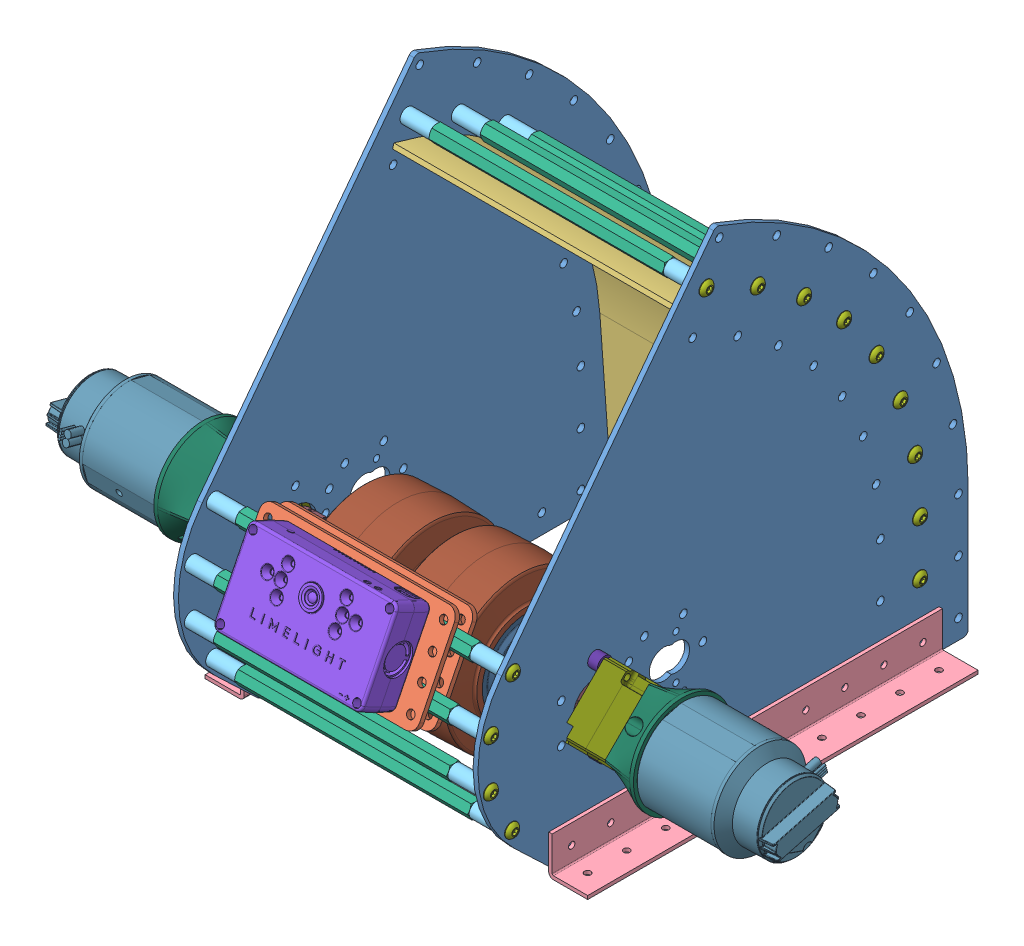
SolidWorks assembly WCP-0281 Rev1 - GreyT Shooter (Falcon VP Direct), configuration Default. Lengths in mm.
Overall size (474.18 324.22 346.91).
112 component instances, 17 part files, 15 mates.
Components (placement in the parent):
- frame-GreyT Shooter (Falcon VP Direct)-1: frame-GreyT Shooter (Falcon VP Direct) [Default] at (99.05 0 0) size (248.9 311.77 324.97)
  - WCP-0281-001 Rev1-1: WCP-0281-001 Rev1 [Default] at (-1.5875 82.55 -30.1625) size (3.17 311.77 319.09)
  - WCP-0281-001 Rev1-2: WCP-0281-001 Rev1 [Default] at (-196.5125 82.55 -30.1625) size (3.17 311.77 319.09)
  - WCP-0281-005 Rev1-1: WCP-0281-005 Rev1 [Default] at (-98.4446 110.2154 24.9678) x (1 0 0) z (0 0.446198 0.894934) size (127 63.5 3.17)
  - WCP-0281-005 Rev1-2: WCP-0281-005 Rev1 [Default] at (-98.4446 115.8821 36.3334) x (1 0 0) z (0 0.446198 0.894934) size (127 63.5 3.17)
  - polycarb_flex_panel (WCP-0281-006) Rev1-1: polycarb_flex_panel (WCP-0281-006) Rev1 [Default] at (-97.1926 99.11 -45.232) x (1 0 0) z (0 -0.072501 0.997368) size (184.15 254.67 126.03)
  - WCP-0281-004 Rev1-1: WCP-0281-004 Rev1 [Default] at (0 0 -114.3) size (25.4 25.4 254)
  - WCP-0281-004 Rev1-2: WCP-0281-004 Rev1 [Default] at (-198.1 0 -139.7) x (-1 0 0) z (0 0 -1) size (25.4 25.4 254)
  - spacer_assembly^frame-GreyT Shooter (Falcon VP Direct)-1: spacer_assembly^frame-GreyT Shooter (Falcon VP Direct) [Default] at (-3.8 277.1819 -108.5961) x (1 0 0) z (0 0.167761 -0.985828) size (204.43 13.43 13.43)
    - WCP-0217 Rev1-1: WCP-0217 Rev1 [Default] at (-180.975 -4.7625 -5.4993) x (1 0 0) z (0 -0.707903 0.70631) size (19.05 9.5 9.5)
    - 91780A094_ALUM FEM THRDED HEX STANDOFF (1)_91780A094-1: 91780A094_ALUM FEM THRDED HEX STANDOFF (1)_91780A094 [Default] at (-95.25 -4.7625 -5.4993) x (0 -1 0) z (-1 0 0) size (9.53 11 152.4)
    - WCP-0217 Rev1-2: WCP-0217 Rev1 [Default] at (-9.525 -4.7625 -5.4993) x (1 0 0) z (0 -0.707903 0.70631) size (19.05 9.5 9.5)
    - WCP-0256 Rev1-1: WCP-0256 Rev1 [Default] at (-196.8654 -4.7625 -5.4993) x (0 -0.959732 -0.280918) z (-1 0 0) size (9.24 9.28 34.97)
    - WCP-0256 Rev1-2: WCP-0256 Rev1 [Default] at (6.3654 -4.7625 -5.4993) x (0 0.566489 -0.82407) z (1 0 0) size (9.24 9.28 34.97)
  - spacer_assembly^frame-GreyT Shooter (Falcon VP Direct)-2: spacer_assembly^frame-GreyT Shooter (Falcon VP Direct) [Default] at (-3.8 258.4844 -133.4749) x (1 0 0) z (0 -0.921698 -0.387907) size (204.43 13.43 13.43)
    - WCP-0217 Rev1-1: WCP-0217 Rev1 [Default] at (-180.975 -4.7625 -5.4993) x (1 0 0) z (0 -0.707903 0.70631) size (19.05 9.5 9.5)
    - 91780A094_ALUM FEM THRDED HEX STANDOFF (1)_91780A094-1: 91780A094_ALUM FEM THRDED HEX STANDOFF (1)_91780A094 [Default] at (-95.25 -4.7625 -5.4993) x (0 -1 0) z (-1 0 0) size (9.53 11 152.4)
    - WCP-0217 Rev1-2: WCP-0217 Rev1 [Default] at (-9.525 -4.7625 -5.4993) x (1 0 0) z (0 -0.707903 0.70631) size (19.05 9.5 9.5)
    - WCP-0256 Rev1-1: WCP-0256 Rev1 [Default] at (-196.8654 -4.7625 -5.4993) x (0 -0.959732 -0.280918) z (-1 0 0) size (9.24 9.28 34.97)
    - WCP-0256 Rev1-2: WCP-0256 Rev1 [Default] at (6.3654 -4.7625 -5.4993) x (0 0.566489 -0.82407) z (1 0 0) size (9.24 9.28 34.97)
  - spacer_assembly^frame-GreyT Shooter (Falcon VP Direct)-3: spacer_assembly^frame-GreyT Shooter (Falcon VP Direct) [Default] at (-3.8 237.3746 -163.6227) x (1 0 0) z (0 -0.921698 -0.387907) size (204.43 13.43 13.43)
    - WCP-0217 Rev1-1: WCP-0217 Rev1 [Default] at (-180.975 -4.7625 -5.4993) x (1 0 0) z (0 -0.707903 0.70631) size (19.05 9.5 9.5)
    - 91780A094_ALUM FEM THRDED HEX STANDOFF (1)_91780A094-1: 91780A094_ALUM FEM THRDED HEX STANDOFF (1)_91780A094 [Default] at (-95.25 -4.7625 -5.4993) x (0 -1 0) z (-1 0 0) size (9.53 11 152.4)
    - WCP-0217 Rev1-2: WCP-0217 Rev1 [Default] at (-9.525 -4.7625 -5.4993) x (1 0 0) z (0 -0.707903 0.70631) size (19.05 9.5 9.5)
    - WCP-0256 Rev1-1: WCP-0256 Rev1 [Default] at (-196.8654 -4.7625 -5.4993) x (0 -0.959732 -0.280918) z (-1 0 0) size (9.24 9.28 34.97)
    - WCP-0256 Rev1-2: WCP-0256 Rev1 [Default] at (6.3654 -4.7625 -5.4993) x (0 0.566489 -0.82407) z (1 0 0) size (9.24 9.28 34.97)
  - spacer_assembly^frame-GreyT Shooter (Falcon VP Direct)-4: spacer_assembly^frame-GreyT Shooter (Falcon VP Direct) [Default] at (-3.8 211.3505 -189.6468) x (1 0 0) z (0 -0.921698 -0.387907) size (204.43 13.43 13.43)
    - WCP-0217 Rev1-1: WCP-0217 Rev1 [Default] at (-180.975 -4.7625 -5.4993) x (1 0 0) z (0 -0.707903 0.70631) size (19.05 9.5 9.5)
    - 91780A094_ALUM FEM THRDED HEX STANDOFF (1)_91780A094-1: 91780A094_ALUM FEM THRDED HEX STANDOFF (1)_91780A094 [Default] at (-95.25 -4.7625 -5.4993) x (0 -1 0) z (-1 0 0) size (9.53 11 152.4)
    - WCP-0217 Rev1-2: WCP-0217 Rev1 [Default] at (-9.525 -4.7625 -5.4993) x (1 0 0) z (0 -0.707903 0.70631) size (19.05 9.5 9.5)
    - WCP-0256 Rev1-1: WCP-0256 Rev1 [Default] at (-196.8654 -4.7625 -5.4993) x (0 -0.959732 -0.280918) z (-1 0 0) size (9.24 9.28 34.97)
    - WCP-0256 Rev1-2: WCP-0256 Rev1 [Default] at (6.3654 -4.7625 -5.4993) x (0 0.566489 -0.82407) z (1 0 0) size (9.24 9.28 34.97)
  - spacer_assembly^frame-GreyT Shooter (Falcon VP Direct)-5: spacer_assembly^frame-GreyT Shooter (Falcon VP Direct) [Default] at (-3.8 181.2027 -210.7566) x (1 0 0) z (0 -0.921698 -0.387907) size (204.43 13.43 13.43)
    - WCP-0217 Rev1-1: WCP-0217 Rev1 [Default] at (-180.975 -4.7625 -5.4993) x (1 0 0) z (0 -0.707903 0.70631) size (19.05 9.5 9.5)
    - 91780A094_ALUM FEM THRDED HEX STANDOFF (1)_91780A094-1: 91780A094_ALUM FEM THRDED HEX STANDOFF (1)_91780A094 [Default] at (-95.25 -4.7625 -5.4993) x (0 -1 0) z (-1 0 0) size (9.53 11 152.4)
    - WCP-0217 Rev1-2: WCP-0217 Rev1 [Default] at (-9.525 -4.7625 -5.4993) x (1 0 0) z (0 -0.707903 0.70631) size (19.05 9.5 9.5)
    - WCP-0256 Rev1-1: WCP-0256 Rev1 [Default] at (-196.8654 -4.7625 -5.4993) x (0 -0.959732 -0.280918) z (-1 0 0) size (9.24 9.28 34.97)
    - WCP-0256 Rev1-2: WCP-0256 Rev1 [Default] at (6.3654 -4.7625 -5.4993) x (0 0.566489 -0.82407) z (1 0 0) size (9.24 9.28 34.97)
  - spacer_assembly^frame-GreyT Shooter (Falcon VP Direct)-6: spacer_assembly^frame-GreyT Shooter (Falcon VP Direct) [Default] at (-3.8 147.8472 -226.3105) x (1 0 0) z (0 -0.921698 -0.387907) size (204.43 13.43 13.43)
    - WCP-0217 Rev1-1: WCP-0217 Rev1 [Default] at (-180.975 -4.7625 -5.4993) x (1 0 0) z (0 -0.707903 0.70631) size (19.05 9.5 9.5)
    - 91780A094_ALUM FEM THRDED HEX STANDOFF (1)_91780A094-1: 91780A094_ALUM FEM THRDED HEX STANDOFF (1)_91780A094 [Default] at (-95.25 -4.7625 -5.4993) x (0 -1 0) z (-1 0 0) size (9.53 11 152.4)
    - WCP-0217 Rev1-2: WCP-0217 Rev1 [Default] at (-9.525 -4.7625 -5.4993) x (1 0 0) z (0 -0.707903 0.70631) size (19.05 9.5 9.5)
    - WCP-0256 Rev1-1: WCP-0256 Rev1 [Default] at (-196.8654 -4.7625 -5.4993) x (0 -0.959732 -0.280918) z (-1 0 0) size (9.24 9.28 34.97)
    - WCP-0256 Rev1-2: WCP-0256 Rev1 [Default] at (6.3654 -4.7625 -5.4993) x (0 0.566489 -0.82407) z (1 0 0) size (9.24 9.28 34.97)
  - spacer_assembly^frame-GreyT Shooter (Falcon VP Direct)-7: spacer_assembly^frame-GreyT Shooter (Falcon VP Direct) [Default] at (-3.8 112.2976 -235.836) x (1 0 0) z (0 -0.921698 -0.387907) size (204.43 13.43 13.43)
    - WCP-0217 Rev1-1: WCP-0217 Rev1 [Default] at (-180.975 -4.7625 -5.4993) x (1 0 0) z (0 -0.707903 0.70631) size (19.05 9.5 9.5)
    - 91780A094_ALUM FEM THRDED HEX STANDOFF (1)_91780A094-1: 91780A094_ALUM FEM THRDED HEX STANDOFF (1)_91780A094 [Default] at (-95.25 -4.7625 -5.4993) x (0 -1 0) z (-1 0 0) size (9.53 11 152.4)
    - WCP-0217 Rev1-2: WCP-0217 Rev1 [Default] at (-9.525 -4.7625 -5.4993) x (1 0 0) z (0 -0.707903 0.70631) size (19.05 9.5 9.5)
    - WCP-0256 Rev1-1: WCP-0256 Rev1 [Default] at (-196.8654 -4.7625 -5.4993) x (0 -0.959732 -0.280918) z (-1 0 0) size (9.24 9.28 34.97)
    - WCP-0256 Rev1-2: WCP-0256 Rev1 [Default] at (6.3654 -4.7625 -5.4993) x (0 0.566489 -0.82407) z (1 0 0) size (9.24 9.28 34.97)
  - spacer_assembly^frame-GreyT Shooter (Falcon VP Direct)-8: spacer_assembly^frame-GreyT Shooter (Falcon VP Direct) [Default] at (-3.8 75.6339 -239.0436) x (1 0 0) z (0 -0.921698 -0.387907) size (204.43 13.43 13.43)
    - WCP-0217 Rev1-1: WCP-0217 Rev1 [Default] at (-180.975 -4.7625 -5.4993) x (1 0 0) z (0 -0.707903 0.70631) size (19.05 9.5 9.5)
    - 91780A094_ALUM FEM THRDED HEX STANDOFF (1)_91780A094-1: 91780A094_ALUM FEM THRDED HEX STANDOFF (1)_91780A094 [Default] at (-95.25 -4.7625 -5.4993) x (0 -1 0) z (-1 0 0) size (9.53 11 152.4)
    - WCP-0217 Rev1-2: WCP-0217 Rev1 [Default] at (-9.525 -4.7625 -5.4993) x (1 0 0) z (0 -0.707903 0.70631) size (19.05 9.5 9.5)
    - WCP-0256 Rev1-1: WCP-0256 Rev1 [Default] at (-196.8654 -4.7625 -5.4993) x (0 -0.959732 -0.280918) z (-1 0 0) size (9.24 9.28 34.97)
    - WCP-0256 Rev1-2: WCP-0256 Rev1 [Default] at (6.3654 -4.7625 -5.4993) x (0 0.566489 -0.82407) z (1 0 0) size (9.24 9.28 34.97)
  - spacer_assembly^frame-GreyT Shooter (Falcon VP Direct)-9: spacer_assembly^frame-GreyT Shooter (Falcon VP Direct) [Default] at (-3.8 40.6593 -243.3983) x (1 0 0) z (0 -0.534977 -0.844867) size (204.43 13.43 13.43)
    - WCP-0217 Rev1-1: WCP-0217 Rev1 [Default] at (-180.975 -4.7625 -5.4993) x (1 0 0) z (0 -0.707903 0.70631) size (19.05 9.5 9.5)
    - 91780A094_ALUM FEM THRDED HEX STANDOFF (1)_91780A094-1: 91780A094_ALUM FEM THRDED HEX STANDOFF (1)_91780A094 [Default] at (-95.25 -4.7625 -5.4993) x (0 -1 0) z (-1 0 0) size (9.53 11 152.4)
    - WCP-0217 Rev1-2: WCP-0217 Rev1 [Default] at (-9.525 -4.7625 -5.4993) x (1 0 0) z (0 -0.707903 0.70631) size (19.05 9.5 9.5)
    - WCP-0256 Rev1-1: WCP-0256 Rev1 [Default] at (-196.8654 -4.7625 -5.4993) x (0 -0.959732 -0.280918) z (-1 0 0) size (9.24 9.28 34.97)
    - WCP-0256 Rev1-2: WCP-0256 Rev1 [Default] at (6.3654 -4.7625 -5.4993) x (0 0.566489 -0.82407) z (1 0 0) size (9.24 9.28 34.97)
  - spacer_assembly^frame-GreyT Shooter (Falcon VP Direct)-13: spacer_assembly^frame-GreyT Shooter (Falcon VP Direct) [Default] at (-3.8 119.8597 24.594) x (1 0 0) z (0 -0.833886 -0.551937) size (204.43 13.43 13.43)
    - WCP-0217 Rev1-1: WCP-0217 Rev1 [Default] at (-180.975 -4.7625 -5.4993) x (1 0 0) z (0 -0.707903 0.70631) size (19.05 9.5 9.5)
    - 91780A094_ALUM FEM THRDED HEX STANDOFF (1)_91780A094-1: 91780A094_ALUM FEM THRDED HEX STANDOFF (1)_91780A094 [Default] at (-95.25 -4.7625 -5.4993) x (0 -1 0) z (-1 0 0) size (9.53 11 152.4)
    - WCP-0217 Rev1-2: WCP-0217 Rev1 [Default] at (-9.525 -4.7625 -5.4993) x (1 0 0) z (0 -0.707903 0.70631) size (19.05 9.5 9.5)
    - WCP-0256 Rev1-1: WCP-0256 Rev1 [Default] at (-196.8654 -4.7625 -5.4993) x (0 -0.959732 -0.280918) z (-1 0 0) size (9.24 9.28 34.97)
    - WCP-0256 Rev1-2: WCP-0256 Rev1 [Default] at (6.3654 -4.7625 -5.4993) x (0 0.566489 -0.82407) z (1 0 0) size (9.24 9.28 34.97)
  - spacer_assembly^frame-GreyT Shooter (Falcon VP Direct)-14: spacer_assembly^frame-GreyT Shooter (Falcon VP Direct) [Default] at (-3.8 91.5232 38.722) x (1 0 0) z (0 -0.833886 -0.551937) size (204.43 13.43 13.43)
    - WCP-0217 Rev1-1: WCP-0217 Rev1 [Default] at (-180.975 -4.7625 -5.4993) x (1 0 0) z (0 -0.707903 0.70631) size (19.05 9.5 9.5)
    - 91780A094_ALUM FEM THRDED HEX STANDOFF (1)_91780A094-1: 91780A094_ALUM FEM THRDED HEX STANDOFF (1)_91780A094 [Default] at (-95.25 -4.7625 -5.4993) x (0 -1 0) z (-1 0 0) size (9.53 11 152.4)
    - WCP-0217 Rev1-2: WCP-0217 Rev1 [Default] at (-9.525 -4.7625 -5.4993) x (1 0 0) z (0 -0.707903 0.70631) size (19.05 9.5 9.5)
    - WCP-0256 Rev1-1: WCP-0256 Rev1 [Default] at (-196.8654 -4.7625 -5.4993) x (0 -0.959732 -0.280918) z (-1 0 0) size (9.24 9.28 34.97)
    - WCP-0256 Rev1-2: WCP-0256 Rev1 [Default] at (6.3654 -4.7625 -5.4993) x (0 0.566489 -0.82407) z (1 0 0) size (9.24 9.28 34.97)
  - spacer_assembly^frame-GreyT Shooter (Falcon VP Direct)-15: spacer_assembly^frame-GreyT Shooter (Falcon VP Direct) [Default] at (-3.8 59.8605 38.8878) x (1 0 0) z (0 -0.833886 -0.551937) size (204.43 13.43 13.43)
    - WCP-0217 Rev1-1: WCP-0217 Rev1 [Default] at (-180.975 -4.7625 -5.4993) x (1 0 0) z (0 -0.707903 0.70631) size (19.05 9.5 9.5)
    - 91780A094_ALUM FEM THRDED HEX STANDOFF (1)_91780A094-1: 91780A094_ALUM FEM THRDED HEX STANDOFF (1)_91780A094 [Default] at (-95.25 -4.7625 -5.4993) x (0 -1 0) z (-1 0 0) size (9.53 11 152.4)
    - WCP-0217 Rev1-2: WCP-0217 Rev1 [Default] at (-9.525 -4.7625 -5.4993) x (1 0 0) z (0 -0.707903 0.70631) size (19.05 9.5 9.5)
    - WCP-0256 Rev1-1: WCP-0256 Rev1 [Default] at (-196.8654 -4.7625 -5.4993) x (0 -0.959732 -0.280918) z (-1 0 0) size (9.24 9.28 34.97)
    - WCP-0256 Rev1-2: WCP-0256 Rev1 [Default] at (6.3654 -4.7625 -5.4993) x (0 0.566489 -0.82407) z (1 0 0) size (9.24 9.28 34.97)
  - spacer_assembly^frame-GreyT Shooter (Falcon VP Direct)-16: spacer_assembly^frame-GreyT Shooter (Falcon VP Direct) [Default] at (-3.8 31.3776 25.0573) x (1 0 0) z (0 -0.833886 -0.551937) size (204.43 13.43 13.43)
    - WCP-0217 Rev1-1: WCP-0217 Rev1 [Default] at (-180.975 -4.7625 -5.4993) x (1 0 0) z (0 -0.707903 0.70631) size (19.05 9.5 9.5)
    - 91780A094_ALUM FEM THRDED HEX STANDOFF (1)_91780A094-1: 91780A094_ALUM FEM THRDED HEX STANDOFF (1)_91780A094 [Default] at (-95.25 -4.7625 -5.4993) x (0 -1 0) z (-1 0 0) size (9.53 11 152.4)
    - WCP-0217 Rev1-2: WCP-0217 Rev1 [Default] at (-9.525 -4.7625 -5.4993) x (1 0 0) z (0 -0.707903 0.70631) size (19.05 9.5 9.5)
    - WCP-0256 Rev1-1: WCP-0256 Rev1 [Default] at (-196.8654 -4.7625 -5.4993) x (0 -0.959732 -0.280918) z (-1 0 0) size (9.24 9.28 34.97)
    - WCP-0256 Rev1-2: WCP-0256 Rev1 [Default] at (6.3654 -4.7625 -5.4993) x (0 0.566489 -0.82407) z (1 0 0) size (9.24 9.28 34.97)
- LimelightCAD2STEPSimp-1: LimelightCAD2STEPSimp [Default] at (9.23 125.4056 67.1857) x (1 0 0) z (0 -0.894934 0.446198) size (97.88 26.09 57.01)
- flywheel_assembly - GreyT Shooter (Falcon VP Direct)-2: flywheel_assembly - GreyT Shooter (Falcon VP Direct) [Default] at (0 84.6779 -8.3849) x (1 0 0) z (0 0.587407 -0.809292) size (127 136.01 136.01)
  - flywheel_bar - GreyT Shooter (Falcon VP Direct)-1: flywheel_bar - GreyT Shooter (Falcon VP Direct) [Default] at (0 14.5144 16.3745) size (127 12.7 13.75)
    - WCP-0281-007 Rev1-1: WCP-0281-007 Rev1 [Default] at origin size (127 12.7 13.75)
  - 2in_flywheel_w_hex (217-4054)-1: 2in_flywheel_w_hex (217-4054) [Default] at (-28.9766 14.5144 16.3598) x (1 0 0) z (0 0.866025 0.5) size (57.95 99.57 99.57)
    - 217-4054-003 Rev1-1: 217-4054-003 Rev1 [Default] at origin size (55.55 82.55 82.55)
    - 217-4054-004 Rev1-1: 217-4054-004 Rev1 [Default] at origin size (50.8 99.57 99.57)
    - 217-4054-002 Rev15-1: 217-4054-002 Rev15 [Default] x (0 0 1) z (-1 0 0) size (50.79 50.79 57.95)
  - 2in_flywheel_w_hex (217-4054)-2: 2in_flywheel_w_hex (217-4054) [Default] at (28.9766 14.5398 16.3745) size (57.95 99.57 99.57)
    - 217-4054-003 Rev1-1: 217-4054-003 Rev1 [Default] at origin size (55.55 82.55 82.55)
    - 217-4054-004 Rev1-1: 217-4054-004 Rev1 [Default] at origin size (50.8 99.57 99.57)
    - 217-4054-002 Rev15-1: 217-4054-002 Rev15 [Default] x (0 0 1) z (-1 0 0) size (50.79 50.79 57.95)
- turret_motor_assembly (Falcon VP Direct)-3: turret_motor_assembly (Falcon VP Direct) [Default] at (-6.975 82.55 -30.1625) x (-1 0 0) z (0 0 -1) size (180.04 90.51 90.51)
  - 217-4008_500_Hex_Coupler-1: 217-4008_500_Hex_Coupler [Default] at (69.85 0 0) x (0 -0.407164 -0.913355) z (1 0 0) size (25.38 22.32 39.56)
  - 217-6515_Falcon_500_Default_As Machined_-1: 217-6515_Falcon_500_Default_As Machined_ [Default] at (175.3 0 0) x (0 0.965926 -0.258819) z (-1 0 0) size (63.31 63.31 115.82)
  - 217-4018_VersaPlanetary_CIM_Adapter-1: 217-4018_VersaPlanetary_CIM_Adapter [Default] at (137.575 0 0) x (0 -0.707107 -0.707107) z (0 0.707107 -0.707107) size (64 21.67 64)
  - v2_versa_planetary_1_stage_no_motor-1: v2_versa_planetary_1_stage_no_motor [Default] at (115.05 -15.7154 15.7154) x (-1 0 0) z (0 -0.707107 -0.707107) size (91.96 44.45 42)
  - WCP-0308-1: WCP-0308 [Default] at (95.25 25.4 0) size (6.35 9.5 9.5)
  - WCP-0308-2: WCP-0308 [Default] at (95.25 -25.4 0) size (6.35 9.5 9.5)
- turret_motor_assembly (Falcon VP Direct)-4: turret_motor_assembly (Falcon VP Direct) [Default] at (6.975 82.55 -30.1625) size (180.04 90.51 90.51)
  - 217-4008_500_Hex_Coupler-1: 217-4008_500_Hex_Coupler [Default] at (69.85 0 0) x (0 -0.407164 -0.913355) z (1 0 0) size (25.38 22.32 39.56)
  - 217-6515_Falcon_500_Default_As Machined_-1: 217-6515_Falcon_500_Default_As Machined_ [Default] at (175.3 0 0) x (0 0.965926 -0.258819) z (-1 0 0) size (63.31 63.31 115.82)
  - 217-4018_VersaPlanetary_CIM_Adapter-1: 217-4018_VersaPlanetary_CIM_Adapter [Default] at (137.575 0 0) x (0 -0.707107 -0.707107) z (0 0.707107 -0.707107) size (64 21.67 64)
  - v2_versa_planetary_1_stage_no_motor-1: v2_versa_planetary_1_stage_no_motor [Default] at (115.05 -15.7154 15.7154) x (-1 0 0) z (0 -0.707107 -0.707107) size (91.96 44.45 42)
  - WCP-0308-1: WCP-0308 [Default] at (95.25 25.4 0) size (6.35 9.5 9.5)
  - WCP-0308-2: WCP-0308 [Default] at (95.25 -25.4 0) size (6.35 9.5 9.5)
Mates (geometry in assembly coordinates):
- Concentric5: concentric aligned: cylinder of frame-GreyT Shooter (Falcon VP Direct)-1/WCP-0281-005 Rev1-1 through (45.0554 130.8177 12.922) axis (0 0.446198 0.894934) radius 2.5527; cylinder of LimelightCAD2STEPSimp-1 through (45.0554 137.9011 27.129) axis (0 0.446198 0.894934) radius 2.5527
- Concentric6: concentric aligned: cylinder of frame-GreyT Shooter (Falcon VP Direct)-1/WCP-0281-005 Rev1-1 through (-43.8446 88.1965 34.1721) axis (0 0.446198 0.894934) radius 2.5527; cylinder of LimelightCAD2STEPSimp-1 through (-43.8446 95.2799 48.3792) axis (0 0.446198 0.894934) radius 2.5527
- Concentric7: concentric aligned: cylinder of frame-GreyT Shooter (Falcon VP Direct)-1/WCP-0281-001 Rev1-1 through (95.875 107.95 -30.1625) axis (1 0 0) radius 2.4892; cylinder of turret_motor_assembly (Falcon VP Direct)-4/v2_versa_planetary_1_stage_no_motor-1 through (122.025 107.95 -30.1625) axis (1 0 0) radius 2.0193
- Concentric8: concentric aligned: cylinder of frame-GreyT Shooter (Falcon VP Direct)-1/WCP-0281-001 Rev1-1 through (95.875 57.15 -30.1625) axis (1 0 0) radius 2.4892; cylinder of turret_motor_assembly (Falcon VP Direct)-4/v2_versa_planetary_1_stage_no_motor-1 through (122.025 57.15 -30.1625) axis (1 0 0) radius 2.0193
- Concentric12: concentric anti-aligned: cylinder of frame-GreyT Shooter (Falcon VP Direct)-1/WCP-0281-001 Rev1-2 through (-99.05 57.15 -30.1625) axis (1 0 0) radius 2.4892; cylinder of turret_motor_assembly (Falcon VP Direct)-3/v2_versa_planetary_1_stage_no_motor-1 through (-122.025 57.15 -30.1625) axis (-1 0 0) radius 2.0193
- Concentric13: concentric anti-aligned: cylinder of frame-GreyT Shooter (Falcon VP Direct)-1/WCP-0281-001 Rev1-2 through (-99.05 107.95 -30.1625) axis (1 0 0) radius 2.4892; cylinder of turret_motor_assembly (Falcon VP Direct)-3/v2_versa_planetary_1_stage_no_motor-1 through (-122.025 107.95 -30.1625) axis (-1 0 0) radius 2.0193
- Concentric14: concentric anti-aligned: cylinder of flywheel_assembly - GreyT Shooter (Falcon VP Direct)-2/flywheel_bar - GreyT Shooter (Falcon VP Direct)-1/WCP-0281-007 Rev1-1 through (57.15 82.55 -30.1625) axis (-1 0 0) radius 2.5527; circle of turret_motor_assembly (Falcon VP Direct)-4/217-4008_500_Hex_Coupler-1
- Coincident6: coincident aligned: plane of frame-GreyT Shooter (Falcon VP Direct)-1 through (0 0 0) normal (1 0 0)
- Coincident7: coincident aligned: plane of frame-GreyT Shooter (Falcon VP Direct)-1/WCP-0281-004 Rev1-2 through (-97.5641 0 0) normal (0 0 1)
- Coincident8: coincident anti-aligned: plane of frame-GreyT Shooter (Falcon VP Direct)-1/WCP-0281-004 Rev1-1 through (99.05 0 -863.6) normal (0 -1 0)
- Coincident9: coincident aligned: plane of flywheel_assembly - GreyT Shooter (Falcon VP Direct)-2 through (0 84.6779 -8.3849) normal (1 0 0)
- Parallel1: parallel anti-aligned: plane of flywheel_assembly - GreyT Shooter (Falcon VP Direct)-2/flywheel_bar - GreyT Shooter (Falcon VP Direct)-1/WCP-0281-007 Rev1-1 through (57.15 88.3498 -32.748) normal (0 0.913355 -0.407164); plane of turret_motor_assembly (Falcon VP Direct)-4/217-4008_500_Hex_Coupler-1 through (57.775 86.8978 -36.1526) normal (0 -0.913355 0.407164)
- Coincident11: coincident anti-aligned: plane of frame-GreyT Shooter (Falcon VP Direct)-1/WCP-0281-005 Rev1-2 through (0.6054 116.5905 37.7541) normal (0 0.446198 0.894934); plane of LimelightCAD2STEPSimp-1 through (0.6054 116.5905 37.7541) normal (0 -0.446198 -0.894934)
- Coincident13: coincident anti-aligned: plane of frame-GreyT Shooter (Falcon VP Direct)-1/WCP-0281-001 Rev1-1 through (99.05 82.55 -30.1625) normal (1 0 0); plane of turret_motor_assembly (Falcon VP Direct)-4/WCP-0308-1 through (99.05 107.95 -30.1625) normal (-1 0 0)
- Coincident14: coincident anti-aligned: plane of frame-GreyT Shooter (Falcon VP Direct)-1/WCP-0281-001 Rev1-2 through (-99.05 82.55 -30.1625) normal (-1 0 0); plane of turret_motor_assembly (Falcon VP Direct)-3/WCP-0308-1 through (-99.05 107.95 -30.1625) normal (1 0 0)
